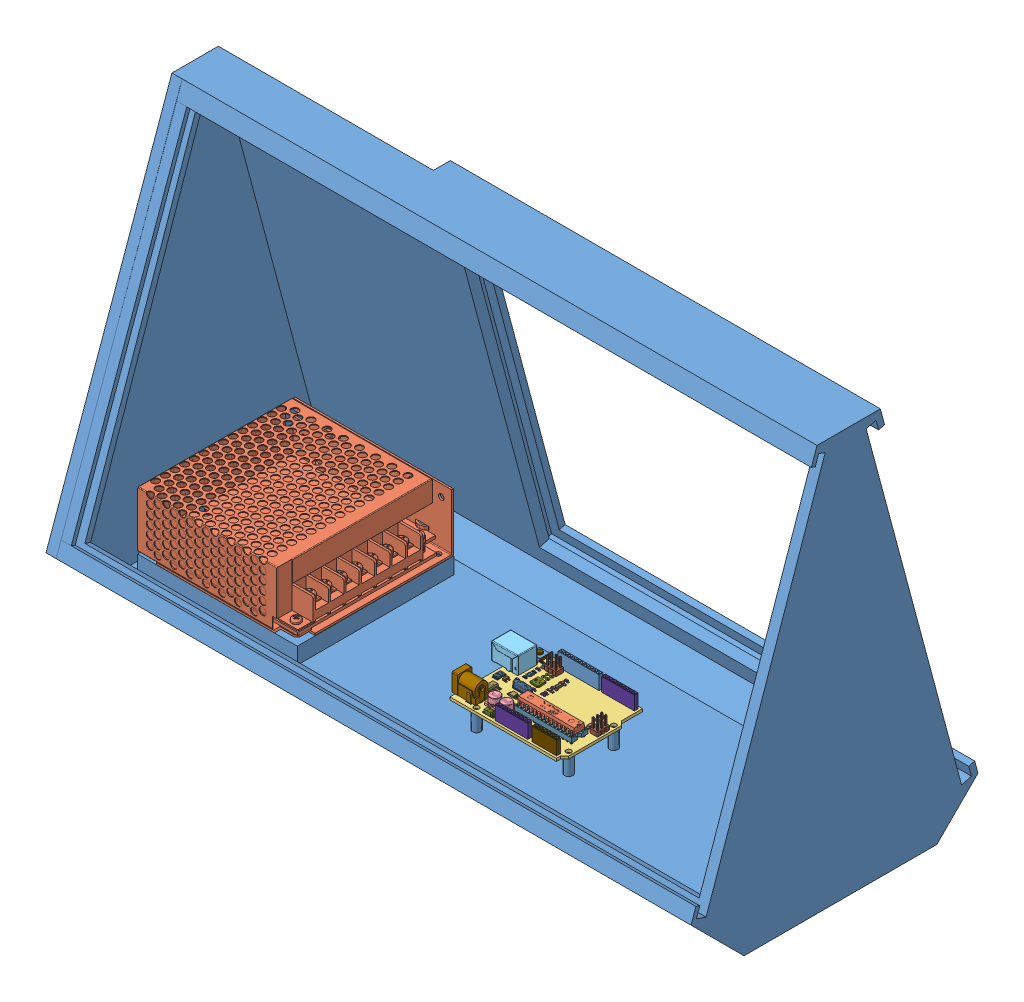
SolidWorks assembly FinalAssembly, configuration Default. Lengths in mm.
Overall size (400.05 251.47 177.92).
87 component instances, 37 part files, 5 mates.
Components (placement in the parent):
- MainBody-1: MainBody [Default] at (286.8797 137.4549 282.9376) size (400.05 251.47 177.92)
- VGD-30-D512-1: VGD-30-D512 [Default] at (-1.4739 148.947 242.9919) x (0.001681 0 -0.999999) z (0.999999 0 0.001681) size (97.06 36.13 99.03)
- arduino uno-1: arduino uno [Default] at (74.7897 150.597 321.5056) x (0 0 1) z (-1 0 0) size (53.34 15.25 74.93)
  - unoboard blue-1: unoboard blue [Default] at origin size (53.34 1.65 68.58)
  - 47uf CAP Dcase-1: 47uf CAP Dcase [Default] at (-9.4141 0 -18.4991) x (0 0 -1) z (1 0 0) size (6.6 5.81 8)
  - USB SHELL-1: USB SHELL [Default] at (-38.02 0.43 6.35) size (13.72 15.2 16.51)
  - USB core-1: USB core [Default] at (-38.02 0.43 6.35) size (11.3 10.68 15.75)
  - usb top contact-1: usb top contact [Default] at (-36.77 6.52 5.97) size (1 9.67 13.76)
  - usb btm contact-1: usb btm contact [Default] at (-36.77 4.84 5.97) size (1 6.84 11.76)
  - usb btm contact-2: usb btm contact [Default] at (-39.27 4.84 5.97) size (1 6.84 11.76)
  - usb top contact-2: usb top contact [Default] at (-39.27 6.52 5.97) size (1 9.67 13.76)
  - power jack-1: power jack [Default] at (-7.675 0 1.905) size (11.2 15.2 15.9)
  - 47uf CAP Dcase-2: 47uf CAP Dcase [Default] at (-9.4141 0 -25.7132) x (0 0 -1) z (1 0 0) size (6.6 5.81 8)
  - crystal-1: crystal [Default] at (-26.162 0 -18.923) x (1 0 0) z (0 0 -1) size (4 5 11)
  - 2pin_header__02-1: 2pin_header__02 [Default] at (-46.23 0 -15.75) size (5 11.75 2.54)
  - nano - reg-1: nano - reg [Default] at (-17.399 0 -7.747) size (6.5 1.69 8.3)
  - led-1: led [Default] at (-34.29 0 -27.94) x (0 0 1) z (-1 0 0) size (4 0.9 1.55)
  - 2pin_header__02-2: 2pin_header__02 [Default] at (-30.43 0 -64.91) x (0 0 1) z (-1 0 0) size (5 11.75 2.54)
  - dip28-1: dip28 [Default] at (-16.383 1.5 -46.355) x (0 0 -1) z (1 0 0) size (35.48 2.8 10.1)
  - dip socket pin-1: dip socket pin [Default] at (-20.193 4.3 -62.865) x (0 0 -1) z (1 0 0) size (1.7 7.37 1.7)
  - dip socket pin-2: dip socket pin [Default] at (-12.573 4.3 -62.865) x (0 0 -1) z (1 0 0) size (1.7 7.37 1.7)
  - dip socket pin-3: dip socket pin [Default] at (-20.193 4.3 -60.325) x (0 0 -1) z (1 0 0) size (1.7 7.37 1.7)
  - dip socket pin-4: dip socket pin [Default] at (-12.573 4.3 -60.325) x (0 0 -1) z (1 0 0) size (1.7 7.37 1.7)
  - dip socket pin-5: dip socket pin [Default] at (-20.193 4.3 -57.785) x (0 0 -1) z (1 0 0) size (1.7 7.37 1.7)
  - dip socket pin-6: dip socket pin [Default] at (-12.573 4.3 -57.785) x (0 0 -1) z (1 0 0) size (1.7 7.37 1.7)
  - dip socket pin-7: dip socket pin [Default] at (-20.193 4.3 -55.245) x (0 0 -1) z (1 0 0) size (1.7 7.37 1.7)
  - dip socket pin-8: dip socket pin [Default] at (-12.573 4.3 -55.245) x (0 0 -1) z (1 0 0) size (1.7 7.37 1.7)
  - dip socket pin-9: dip socket pin [Default] at (-20.193 4.3 -52.705) x (0 0 -1) z (1 0 0) size (1.7 7.37 1.7)
  - dip socket pin-10: dip socket pin [Default] at (-12.573 4.3 -52.705) x (0 0 -1) z (1 0 0) size (1.7 7.37 1.7)
  - dip socket pin-11: dip socket pin [Default] at (-20.193 4.3 -50.165) x (0 0 -1) z (1 0 0) size (1.7 7.37 1.7)
  - dip socket pin-12: dip socket pin [Default] at (-12.573 4.3 -50.165) x (0 0 -1) z (1 0 0) size (1.7 7.37 1.7)
  - dip socket pin-13: dip socket pin [Default] at (-20.193 4.3 -47.625) x (0 0 -1) z (1 0 0) size (1.7 7.37 1.7)
  - dip socket pin-14: dip socket pin [Default] at (-12.573 4.3 -47.625) x (0 0 -1) z (1 0 0) size (1.7 7.37 1.7)
  - dip socket pin-15: dip socket pin [Default] at (-20.193 4.3 -45.085) x (0 0 -1) z (1 0 0) size (1.7 7.37 1.7)
  - dip socket pin-16: dip socket pin [Default] at (-12.573 4.3 -45.085) x (0 0 -1) z (1 0 0) size (1.7 7.37 1.7)
  - dip socket pin-17: dip socket pin [Default] at (-20.193 4.3 -42.545) x (0 0 -1) z (1 0 0) size (1.7 7.37 1.7)
  - dip socket pin-18: dip socket pin [Default] at (-12.573 4.3 -42.545) x (0 0 -1) z (1 0 0) size (1.7 7.37 1.7)
  - dip socket pin-19: dip socket pin [Default] at (-20.193 4.3 -40.005) x (0 0 -1) z (1 0 0) size (1.7 7.37 1.7)
  - dip socket pin-20: dip socket pin [Default] at (-12.573 4.3 -40.005) x (0 0 -1) z (1 0 0) size (1.7 7.37 1.7)
  - dip socket pin-21: dip socket pin [Default] at (-20.193 4.3 -37.465) x (0 0 -1) z (1 0 0) size (1.7 7.37 1.7)
  - dip socket pin-22: dip socket pin [Default] at (-12.573 4.3 -37.465) x (0 0 -1) z (1 0 0) size (1.7 7.37 1.7)
  - dip socket pin-23: dip socket pin [Default] at (-20.193 4.3 -34.925) x (0 0 -1) z (1 0 0) size (1.7 7.37 1.7)
  - dip socket pin-24: dip socket pin [Default] at (-12.573 4.3 -34.925) x (0 0 -1) z (1 0 0) size (1.7 7.37 1.7)
  - dip socket pin-25: dip socket pin [Default] at (-20.193 4.3 -32.385) x (0 0 -1) z (1 0 0) size (1.7 7.37 1.7)
  - dip socket pin-26: dip socket pin [Default] at (-12.573 4.3 -32.385) x (0 0 -1) z (1 0 0) size (1.7 7.37 1.7)
  - dip socket pin-27: dip socket pin [Default] at (-20.193 4.3 -29.845) x (0 0 -1) z (1 0 0) size (1.7 7.37 1.7)
  - dip socket pin-28: dip socket pin [Default] at (-12.573 4.3 -29.845) x (0 0 -1) z (1 0 0) size (1.7 7.37 1.7)
  - 2pin_header__02-3: 2pin_header__02 [Default] at (-27.89 0 -64.91) x (0 0 1) z (-1 0 0) size (5 11.75 2.54)
  - 2pin_header__02-4: 2pin_header__02 [Default] at (-25.35 0 -64.91) x (0 0 1) z (-1 0 0) size (5 11.75 2.54)
  - 2pin_header__02-5: 2pin_header__02 [Default] at (-46.23 0 -18.29) size (5 11.75 2.54)
  - 2pin_header__02-6: 2pin_header__02 [Default] at (-46.23 0 -20.83) size (5 11.75 2.54)
  - atmega16u2-1: atmega16u2 [Default] at (-34.671 0.06 -20) x (1 0 0) z (0 0 -1) size (5.5 1.01 5.5)
  - led-2: led [Default] at (-36.83 0 -27.94) x (0 0 1) z (-1 0 0) size (4 0.9 1.55)
  - led-3: led [Default] at (-42.037 0 -27.94) x (0 0 1) z (-1 0 0) size (4 0.9 1.55)
  - led-4: led [Default] at (-36.576 0 -58.42) x (0 0 1) z (-1 0 0) size (4 0.9 1.55)
  - 8 PORT HEADER-1: 8 PORT HEADER [Default] at (-50.8 0 -45.72) x (0 0 -1) z (1 0 0) size (20.32 10.51 2.41)
  - 8 PORT HEADER-2: 8 PORT HEADER [Default] at (-2.54 0 -27.94) x (0 0 -1) z (1 0 0) size (20.32 10.51 2.41)
  - 6 PORT HEADER-1: 6 PORT HEADER [Default] at (-2.54 0 -50.8) x (0 0 -1) z (1 0 0) size (15.24 10.51 2.41)
  - 10 PORT HEADER-1: 10 PORT HEADER [Default] at (-50.8 0 -18.796) x (0 0 -1) z (1 0 0) size (25.4 10.51 2.41)
  - ATMEL328P-1: ATMEL328P [Default] at (-16.383 4.3 -46.355) x (0 0 -1) z (1 0 0) size (35 7.27 7.87)
  - 102 RESISTOR PACK-1: 102 RESISTOR PACK [Default] at (-33.782 0 -58.42) size (3.2 0.51 3)
  - 102 RESISTOR PACK-2: 102 RESISTOR PACK [Default] at (-39.37 0 -27.94) size (3.2 0.51 3)
  - 103 RESISTOR PACK-1: 103 RESISTOR PACK [Default] at (-23.876 0 -27.94) size (3.2 0.51 3)
  - 220 RESISTOR PACK-1: 220 RESISTOR PACK [Default] at (-36.83 0 -12.827) size (3.2 0.51 3)
  - 16mhz crystal - measured-1: 16mhz crystal - measured [Default] at (-24.892 0 -41.275) x (0 0 -1) z (1 0 0) size (3.4 0.8 2)
  - PADS001-1: PADS001 [Default] at (-39.878 0.1 -18.288) x (-1 0 0) z (0 0 1) size (4.54 0.1 4.54)
  - 603 cap on pad-1: 603 cap on pad [Default] at (-44.45 0 -27.94) x (0 0 -1) z (1 0 0) size (2.76 0.91 1.02)
  - ssot3-1: ssot3 [Default] at (-26.5 0 -8.128) x (-1 0 0) z (0 0 -1) size (3 1.13 3.09)
  - mf-msmf050-2-1: mf-msmf050-2 [Default] at (-26.5 0 -4.064) size (5.76 1.02 3.72)
  - 603 cap on pad-2: 603 cap on pad [Default] at (-29.845 0 -27.94) x (0 0 -1) z (1 0 0) size (2.76 0.91 1.02)
  - 603 cap on pad-3: 603 cap on pad [Default] at (-31.496 0 -27.94) x (0 0 -1) z (1 0 0) size (2.76 0.91 1.02)
  - lmv358-1: lmv358 [Default] at (-15.24 0 -21.971) x (0 0 -1) z (1 0 0) size (3.7 1.4 2.9)
  - 603 cap on pad-4: 603 cap on pad [Default] at (-15.24 0 -18.415) size (2.76 0.91 1.02)
  - 603 cap on pad-5: 603 cap on pad [Default] at (-29.845 0 -12.065) x (0 0 1) z (-1 0 0) size (2.76 0.91 1.02)
  - 603 cap on pad-6: 603 cap on pad [Default] at (-29.591 0 -22.352) x (0 0 1) z (-1 0 0) size (2.76 0.91 1.02)
  - 603 cap on pad-7: 603 cap on pad [Default] at (-29.591 0 -16.002) x (0 0 1) z (-1 0 0) size (2.76 0.91 1.02)
  - 603 cap on pad-8: 603 cap on pad [Default] at (-41.91 0 -12.7) x (0 0 1) z (-1 0 0) size (2.76 0.91 1.02)
  - lp2985dgkr-1: lp2985dgkr [Default] at (-20.32 0 -19.05) x (0 0 -1) z (1 0 0) size (5.85 1.1 3)
  - cd1206 diode-1: cd1206 diode [Default] at (-27.94 0 -59.436) x (0 0 -1) z (1 0 0) size (2.09 0.96 5)
  - cd1206 diode-2: cd1206 diode [Default] at (-46.228 0 -13.081) x (0 0 1) z (-1 0 0) size (2.09 0.96 5)
  - 603 resistor-1: 603 resistor [Default] at (-29.591 0 -19.05) x (0 0 1) z (-1 0 0) size (2.36 0.62 1.03)
  - blm21-1: blm21 [Default] at (-45.085 0 -7.62) x (0 0 -1) z (1 0 0) size (2.78 0.95 1.32)
  - m7 diode-1: m7 diode [Default] at (-2.794 0 -21.59) x (0 0 -1) z (1 0 0) size (6.66 2.35 2.5)
  - MLC0603-1: MLC0603 [Default] at (-33.655 0 -12.827) x (0 0 -1) z (1 0 0) size (2.36 0.6 1.03)
  - MLC0603-2: MLC0603 [Default] at (-39.37 0 -12.827) x (0 0 -1) z (1 0 0) size (2.36 0.6 1.03)
  - RESET CORE-1: RESET CORE [Default] at (-49.403 0.1 -6.35) x (-1 0 0) z (0 0 -1) size (6.2 3.1 9.6)
  - RESET-1: RESET [Default] at (-49.403 0.1 -6.35) x (0 0 1) z (-1 0 0) size (7.3 2 6.2)
Mates (geometry in assembly coordinates):
- Coincident1: coincident anti-aligned: plane of MainBody-1 through (286.8797 148.947 282.9376) normal (0 1 0); plane of VGD-30-D512-1 through (-99.9756 148.947 243.9763) normal (0 -1 0)
- Concentric2: concentric anti-aligned: circle of MainBody-1; circle of VGD-30-D512-1
- Coincident7: coincident: plane of MainBody-1 through (88.7597 148.947 318.9656) normal (0 1 0); plane of arduino uno-1/unoboard blue-1 through (81.3024 148.947 257.9564) normal (0 -1 0)
- Concentric7: concentric: circle of MainBody-1; circle of arduino uno-1/unoboard blue-1
- Concentric9: concentric aligned: circle of MainBody-1; circle of arduino uno-1/unoboard blue-1
